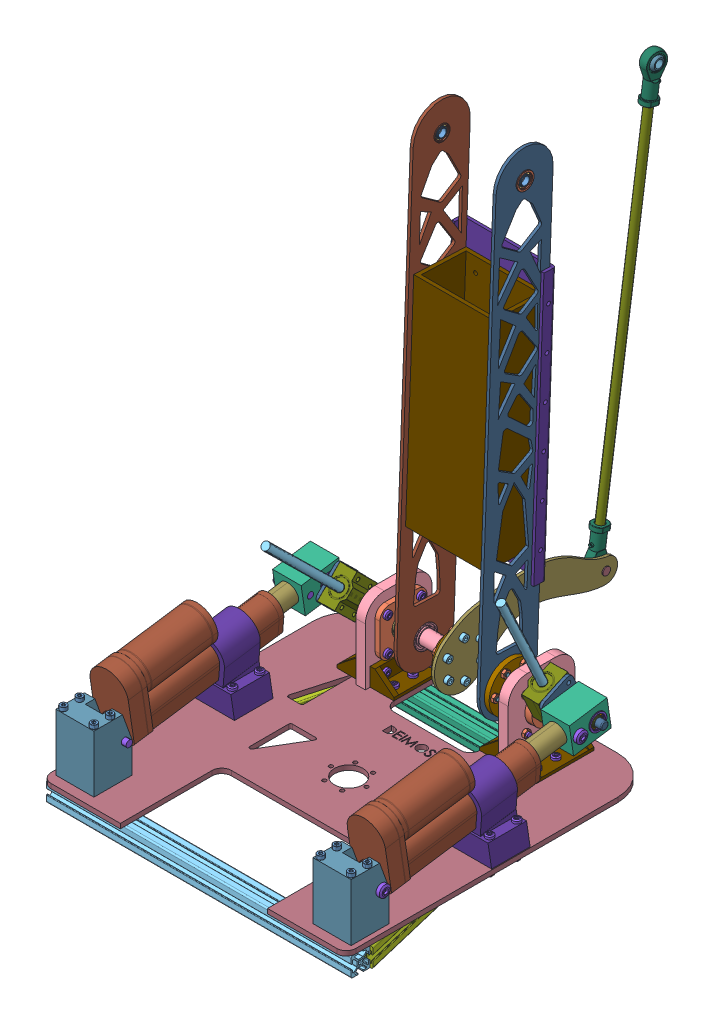
SolidWorks assembly Base + Link1 Final assembly, configuration Default. Lengths in mm. (continued)
Components (placement in the parent): (continued)
- socket head cap screw_iso-13: socket head cap screw_iso [ISO 4762 M4 x 12 - 12N] at (285.0714 147.0946 166.2039) x (-1 0 0) z (0 0.924225 0.381849) size (16 7 7)
- hex nut style 1 gradeab_iso-50: hex nut style 1 gradeab_iso [ISO - 4032 - M4 - W - N] at (269.8714 148.1762 131.5798) x (0 0 1) z (-1 0 0) size (7 8.08 3.2)
- hex nut style 1 gradeab_iso-51: hex nut style 1 gradeab_iso [ISO - 4032 - M4 - W - N] at (269.8714 157.6305 149.2041) x (0 0 1) z (-1 0 0) size (7 8.08 3.2)
- hex nut style 1 gradeab_iso-52: hex nut style 1 gradeab_iso [ISO - 4032 - M4 - W - N] at (269.8714 147.0946 166.2039) x (0 0 1) z (-1 0 0) size (7 8.08 3.2)
- hex nut style 1 gradeab_iso-53: hex nut style 1 gradeab_iso [ISO - 4032 - M4 - W - N] at (269.8714 127.1043 165.5794) x (0 0 1) z (-1 0 0) size (7 8.08 3.2)
- hex nut style 1 gradeab_iso-54: hex nut style 1 gradeab_iso [ISO - 4032 - M4 - W - N] at (269.8714 117.65 147.9551) x (0 0 1) z (-1 0 0) size (7 8.08 3.2)
- hex nut style 1 gradeab_iso-55: hex nut style 1 gradeab_iso [ISO - 4032 - M4 - W - N] at (269.8714 128.186 130.9553) x (0 0 1) z (-1 0 0) size (7 8.08 3.2)
- hex nut style 1 gradeab_iso-56: hex nut style 1 gradeab_iso [ISO - 4032 - M4 - W - N] at (336.7714 154.5674 137.9272) x (0 0 -1) z (1 0 0) size (7 8.08 3.2)
- hex nut style 1 gradeab_iso-57: hex nut style 1 gradeab_iso [ISO - 4032 - M4 - W - N] at (336.7714 136.8786 128.5941) x (0 0 -1) z (1 0 0) size (7 8.08 3.2)
- hex nut style 1 gradeab_iso-58: hex nut style 1 gradeab_iso [ISO - 4032 - M4 - W - N] at (336.7714 155.329 157.9127) x (0 0 -1) z (1 0 0) size (7 8.08 3.2)
- hex nut style 1 gradeab_iso-59: hex nut style 1 gradeab_iso [ISO - 4032 - M4 - W - N] at (336.7714 119.9515 139.2465) x (0 0 -1) z (1 0 0) size (7 8.08 3.2)
- hex nut style 1 gradeab_iso-60: hex nut style 1 gradeab_iso [ISO - 4032 - M4 - W - N] at (336.7714 120.7132 159.232) x (0 0 -1) z (1 0 0) size (7 8.08 3.2)
- hex nut style 1 gradeab_iso-61: hex nut style 1 gradeab_iso [ISO - 4032 - M4 - W - N] at (336.7714 138.4019 168.5651) x (0 0 -1) z (1 0 0) size (7 8.08 3.2)
Mates (geometry in assembly coordinates):
- Coincident12: coincident anti-aligned: plane of V8_base plate for LAURC 2024_V4-1 through (283.5714 92.6403 412.2334) normal (0 1 0); plane of LA_back holder-1 through (148.5714 92.6403 403.5796) normal (0 -1 0)
- Concentric4: concentric anti-aligned: cylinder of Connector to Linear bearing-1/V8_F688ZZ_assemblyURC 2024_V4-2/V8_F688ZZ_shaftURC 2024_V4-1 through (137.4714 160.303 171.5672) axis (-1 0 0) radius 4; cylinder of V8_bearing and cam connection_for_v4URC 2024_V4 laser cut-1 through (125.6714 160.303 171.5672) axis (1 0 0) radius 4
- Distance6: distance = 20 mm: cylinder of Connector to Linear bearing-1/V8_connectorURC 2024_V4-1 through (168.5714 167.5156 156.635) axis (0 -0.146923 0.989148) radius 13; plane of V8_bearing and cam connection_for_v4URC 2024_V4-1 through (188.5714 161.6723 163.3962) normal (-1 0 0)
- Concentric7: concentric aligned: cylinder of V8_LA_Body_V4-1 through (148.5714 127.7454 390.7229) axis (0 0.146946 -0.989144) radius 10; cylinder of V8_LA_RodURC 2024_V4-1 through (148.5714 140.671 303.7169) axis (0 0.146946 -0.989144) radius 10
- Parallel7: parallel aligned: plane of V8_bearing and cam connection_for_v4URC 2024_V4 laser cut-1 through (170.6714 137.31 173.1714) normal (-1 0 0); plane of V8_base plate for LAURC 2024_V4-1 through (123.5714 92.6403 412.2334) normal (-1 0 0)
- Coincident16: coincident anti-aligned: plane of V8_LA_Body_V4-1 through (139.5714 133.2418 401.3618) normal (-1 0 0); plane of LA_back holder-1 through (139.5714 102.6403 403.5796) normal (1 0 0)
- Concentric13: concentric aligned: cylinder of V8_LA_Body_V4-1 through (166.0567 127.6403 391.4309) axis (-1 0 0) radius 3; cylinder of LA_back holder-1 through (196.5714 127.6403 391.4309) axis (-1 0 0) radius 3
- Concentric14: concentric aligned: cylinder of linnear rod coupler-1 through (184.8714 146.065 157.125) axis (0 -0.702057 -0.712121) radius 4; cylinder of linear guid rod-1 through (184.8714 247.1612 259.6704) axis (0 -0.702057 -0.712121) radius 4
- Concentric15: concentric: cylinder of base bearing assambly-1/base shaft bearing housing-1 through (214.5714 142.6403 150.9703) axis (-1 0 0) radius 17; cylinder of V8_bearing holder holderURC 2024_V4-1 through (223.5714 142.6403 150.9703) axis (1 0 0) radius 17.5
- Coincident19: coincident anti-aligned: plane of V8_bearing holder holderURC 2024_V4-1 through (203.5714 92.6403 113.5796) normal (0 -1 0); plane of V8_base plate for LAURC 2024_V4-1 through (283.5714 92.6403 412.2334) normal (0 1 0)
- Concentric21: concentric aligned: cylinder of V8_LA_Body_V4-1 through (166.0567 127.6403 391.4309) axis (-1 0 0) radius 3; cylinder of LA_back holder-1 through (196.5714 127.6403 391.4309) axis (-1 0 0) radius 3
- Concentric24: concentric anti-aligned: cylinder of V8_base plate for LAURC 2024_V4-1 through (132.5714 82.6403 419.5796) axis (0 1 0) radius 2; cylinder of LA_back holder-1 through (132.5714 180.6403 419.5796) axis (0 -1 0) radius 2
- Concentric25: concentric anti-aligned: cylinder of V8_base plate for LAURC 2024_V4-1 through (164.5714 82.6403 419.5796) axis (0 1 0) radius 2; cylinder of LA_back holder-1 through (164.5714 180.6403 419.5796) axis (0 -1 0) radius 2
- Concentric26: concentric aligned: cylinder of Connector to Linear bearing-2/V8_F688ZZ_assemblyURC 2024_V4-2/V8_F688ZZ_shaftURC 2024_V4-1 through (407.4714 162.026 159.969) axis (-1 0 0) radius 4; cylinder of V8_bearing and cam connection_for_v4URC 2024_V4 laser cut-2 through (441.4714 162.026 159.969) axis (-1 0 0) radius 4
- Concentric31: concentric aligned: cylinder of V8_LA_RodURC 2024_V4-2 through (418.5714 142.394 292.1187) axis (0 0.146946 -0.989144) radius 10; cylinder of V8_LA_Body_V4-2 through (418.5714 127.7454 390.7229) axis (0 0.146946 -0.989144) radius 10
- Concentric36: concentric aligned: cylinder of linnear rod coupler-2 through (382.2714 148.5129 153.6577) axis (0 -0.906049 -0.423172) radius 4; cylinder of linear guid rod-2 through (382.2714 269.4957 210.1629) axis (0 -0.906049 -0.423172) radius 4
- Concentric37: concentric anti-aligned: cylinder of base bearing assambly-2/base shaft bearing housing-1 through (370.5714 137.6403 148.5796) axis (1 0 0) radius 17; cylinder of V8_bearing holder holderURC 2024_V4-2 through (363.5714 137.6403 148.5796) axis (-1 0 0) radius 17.5
- Coincident30: coincident anti-aligned: plane of linnear rod coupler-2 through (396.2714 137.6403 148.5796) normal (1 0 0); plane of lock_nut_for coupler-2 through (396.2714 137.6403 148.5796) normal (-1 0 0)
- Coincident31: coincident anti-aligned: plane of V8_base plate for LAURC 2024_V4-1 through (283.5714 92.6403 412.2334) normal (0 1 0); plane of LA_back holder-2 through (418.5714 92.6403 403.5796) normal (0 -1 0)
- Parallel13: parallel aligned: plane of V8_base plate for LAURC 2024_V4-1 through (443.5714 92.6403 412.2334) normal (1 0 0); plane of V8_bearing and cam connection_for_v4URC 2024_V4 laser cut-2 through (396.4714 168.2112 182.1724) normal (1 0 0)
- Coincident32: coincident anti-aligned: plane of V8_base plate for LAURC 2024_V4-1 through (283.5714 92.6403 412.2334) normal (0 1 0); plane of V8_bearing holder holderURC 2024_V4-2 through (363.5714 92.6403 183.5796) normal (0 -1 0)
- Concentric42: concentric anti-aligned: cylinder of V8_base plate for LAURC 2024_V4-1 through (402.5714 82.6403 419.5796) axis (0 1 0) radius 2; cylinder of LA_back holder-2 through (402.5714 180.6403 419.5796) axis (0 -1 0) radius 2
- Concentric43: concentric anti-aligned: cylinder of V8_base plate for LAURC 2024_V4-1 through (434.5714 82.6403 419.5796) axis (0 1 0) radius 2; cylinder of LA_back holder-2 through (434.5714 180.6403 419.5796) axis (0 -1 0) radius 2
- Coincident41: coincident anti-aligned: plane of LA_back holder-2 through (427.5714 102.6403 403.5796) normal (-1 0 0); plane of V8_LA_Body_V4-2 through (427.5714 133.2418 401.3618) normal (1 0 0)
- Concentric60: concentric aligned: cylinder of LA_back holder-2 through (466.5714 127.6403 391.4309) axis (-1 0 0) radius 3; cylinder of V8_LA_Body_V4-2 through (436.0567 127.6403 391.4309) axis (-1 0 0) radius 3
- Coincident46: coincident anti-aligned: plane of V8_bearing and cam connection_for_v4URC 2024_V4 laser cut-2 through (393.4714 168.2112 182.1724) normal (-1 0 0); plane of linear bearing robotic arm-2 through (393.4714 185.0413 170.7184) normal (1 0 0)
- Concentric65: concentric anti-aligned: cylinder of V8_bearing and cam connection_for_v4URC 2024_V4 laser cut-2 through (403.4714 148.7935 167.033) axis (-1 0 0) radius 2; cylinder of linear bearing robotic arm-2 through (385.4714 148.7935 167.033) axis (1 0 0) radius 1.7
- Concentric66: concentric anti-aligned: cylinder of V8_bearing and cam connection_for_v4URC 2024_V4 laser cut-2 through (403.4714 165.1024 174.6501) axis (-1 0 0) radius 2; cylinder of linear bearing robotic arm-2 through (385.4714 165.1024 174.6501) axis (1 0 0) radius 1.7
- Coincident47: coincident anti-aligned: plane of V8_bearing and cam connection_for_v4URC 2024_V4 laser cut-1 through (173.6714 137.31 173.1714) normal (1 0 0); plane of linear bearing robotic arm-1 through (173.6714 142.4694 153.478) normal (-1 0 0)
- Concentric67: concentric aligned: cylinder of V8_bearing and cam connection_for_v4URC 2024_V4 laser cut-1 through (163.6714 175.167 169.5516) axis (1 0 0) radius 2; cone of linear bearing robotic arm-1 through (173.7714 175.167 169.5516) axis (1 0 0)
- Concentric68: concentric aligned: cylinder of V8_bearing and cam connection_for_v4URC 2024_V4 laser cut-1 through (163.6714 162.5299 156.7334) axis (1 0 0) radius 2; cone of linear bearing robotic arm-1 through (173.7714 162.5299 156.7334) axis (1 0 0)
- Concentric69: concentric anti-aligned: cylinder of linear guid rod-2 through (382.2714 269.4957 210.1629) axis (0 -0.906049 -0.423172) radius 4; cylinder of linear bearing robotic arm-2 through (382.2714 148.4352 153.6214) axis (0 0.906049 0.423172) radius 4
- Concentric70: concentric aligned: cylinder of linear guid rod-1 through (184.8714 247.1612 259.6704) axis (0 -0.702057 -0.712121) radius 4; cylinder of linear bearing robotic arm-1 through (184.8714 170.8339 182.249) axis (0 -0.702057 -0.712121) radius 4
- Concentric73: concentric anti-aligned: cylinder of V8_LA_Body_V4-2 through (418.5714 153.3559 218.3306) axis (0 -0.146946 0.989144) radius 14.0003; cylinder of linear_acutator_holder-1 through (418.5714 143.3537 285.6586) axis (0 0.146946 -0.989144) radius 13.9658
- Concentric74: concentric anti-aligned: cylinder of Connector to Linear bearing-2/V8_connectorURC 2024_V4-1 through (418.5714 160.1892 172.3333) axis (0 -0.146946 0.989144) radius 10; cylinder of V8_LA_RodURC 2024_V4-2 through (418.5714 142.394 292.1187) axis (0 0.146946 -0.989144) radius 10
- Concentric76: concentric anti-aligned: cylinder of Connector to Linear bearing-2/V8_connectorURC 2024_V4-1 through (504.5714 159.1459 179.3562) axis (-1 0 0) radius 3; cylinder of V8_LA_RodURC 2024_V4-2 through (408.5704 159.1459 179.3562) axis (1 0 0) radius 3
- Concentric77: concentric anti-aligned: cylinder of Connector to Linear bearing-1/V8_connectorURC 2024_V4-1 through (148.5714 158.4662 183.9315) axis (0 -0.146946 0.989144) radius 10; cylinder of V8_LA_RodURC 2024_V4-1 through (148.5714 140.671 303.7169) axis (0 0.146946 -0.989144) radius 10
- Concentric78: concentric anti-aligned: cylinder of Connector to Linear bearing-1/V8_connectorURC 2024_V4-1 through (234.5714 157.4228 190.9544) axis (-1 0 0) radius 3; cylinder of V8_LA_RodURC 2024_V4-1 through (138.5704 157.4228 190.9544) axis (1 0 0) radius 3
- Coincident51: coincident anti-aligned: plane of V8_base plate for LAURC 2024_V4-1 through (283.5714 92.6403 412.2334) normal (0 1 0); plane of linear_acutator_holder-2 through (124.6971 92.6403 239.7077) normal (0 -1 0)
- Concentric79: concentric anti-aligned: cylinder of V8_LA_Body_V4-1 through (148.5714 153.3559 218.3306) axis (0 -0.146946 0.989144) radius 14.0003; cylinder of linear_acutator_holder-2 through (148.5714 143.3537 285.6586) axis (0 0.146946 -0.989144) radius 18.9535
- Concentric80: concentric anti-aligned: cylinder of base bearing assambly-2/base shaft bearing housing-1 through (358.5714 155.1403 131.0796) axis (-1 0 0) radius 2; cylinder of V8_bearing holder holderURC 2024_V4-2 through (353.5714 155.1403 131.0796) axis (1 0 0) radius 2
- Coincident52: coincident anti-aligned: plane of V8_bearing holder holderURC 2024_V4-2 through (363.5714 172.6403 183.5796) normal (1 0 0); plane of l bracket_arm base flang-1 through (363.5714 111.6403 178.5796) normal (-1 0 0)
- Coincident53: coincident anti-aligned: plane of V8_base plate for LAURC 2024_V4-1 through (283.5714 92.6403 412.2334) normal (0 1 0); plane of l bracket_arm base flang-1 through (368.5714 92.6403 178.5796) normal (0 -1 0)
- Width1: width anti-aligned: plane of l bracket_arm base flang-1 through (368.5714 111.6403 178.5796) normal (0 0 1); plane of V8_bearing holder holderURC 2024_V4-2 through (368.5714 111.6403 118.5796) normal (0 0 -1); plane of l bracket_arm base flang-1 through (363.5714 172.6403 113.5796) normal (0 0 -1); plane of V8_bearing holder holderURC 2024_V4-2 through (363.5714 172.6403 183.5796) normal (0 0 1)
- Coincident55: coincident anti-aligned: plane of V8_base plate for LAURC 2024_V4-1 through (283.5714 92.6403 412.2334) normal (0 1 0); plane of l bracket_arm base flang-2 through (348.5714 92.6403 118.5796) normal (0 -1 0)
- Coincident56: coincident anti-aligned: plane of V8_bearing holder holderURC 2024_V4-2 through (353.5714 172.6403 183.5796) normal (-1 0 0); plane of l bracket_arm base flang-2 through (353.5714 111.6403 118.5796) normal (1 0 0)
- Coincident57: coincident aligned: plane of l bracket_arm base flang-1 through (368.5714 111.6403 118.5796) normal (0 0 -1); plane of l bracket_arm base flang-2 through (348.5714 111.6403 118.5796) normal (0 0 -1)
- Concentric81: concentric anti-aligned: cylinder of base bearing assambly-2/base shaft bearing housing-1 through (370.5714 137.6403 148.5796) axis (1 0 0) radius 17; cylinder of V8_bearing holder holderURC 2024_V4-2 through (363.5714 137.6403 148.5796) axis (-1 0 0) radius 17.5
- Coincident59: coincident anti-aligned: plane of base bearing assambly-2/base shaft bearing housing-1 through (353.5714 172.6403 148.5796) normal (1 0 0); plane of V8_bearing holder holderURC 2024_V4-2 through (353.5714 172.6403 183.5796) normal (-1 0 0)
- Concentric83: concentric anti-aligned: cylinder of base bearing assambly-1/base shaft bearing housing-1 through (196.5714 137.6403 148.5796) axis (-1 0 0) radius 17; cylinder of V8_bearing holder holderURC 2024_V4-1 through (203.5714 137.6403 148.5796) axis (1 0 0) radius 17.5
- Coincident60: coincident aligned: plane of l bracket_arm base flang-2 through (348.5714 111.6403 118.5796) normal (0 0 -1); plane of l bracket_arm base flang-4 through (218.5714 111.6403 118.5796) normal (0 0 -1)
- Coincident61: coincident anti-aligned: plane of V8_bearing holder holderURC 2024_V4-1 through (213.5714 172.6403 113.5796) normal (1 0 0); plane of l bracket_arm base flang-4 through (213.5714 111.6403 178.5796) normal (-1 0 0)
- Coincident62: coincident anti-aligned: plane of V8_base plate for LAURC 2024_V4-1 through (283.5714 92.6403 412.2334) normal (0 1 0); plane of l bracket_arm base flang-4 through (218.5714 92.6403 178.5796) normal (0 -1 0)
- Coincident63: coincident anti-aligned: plane of V8_bearing holder holderURC 2024_V4-1 through (203.5714 172.6403 113.5796) normal (-1 0 0); plane of l bracket_arm base flang-3 through (203.5714 111.6403 118.5796) normal (1 0 0)
- Coincident64: coincident anti-aligned: plane of V8_base plate for LAURC 2024_V4-1 through (283.5714 92.6403 412.2334) normal (0 1 0); plane of l bracket_arm base flang-3 through (198.5714 92.6403 118.5796) normal (0 -1 0)
- Coincident65: coincident aligned: plane of l bracket_arm base flang-3 through (198.5714 111.6403 118.5796) normal (0 0 -1); plane of l bracket_arm base flang-4 through (218.5714 111.6403 118.5796) normal (0 0 -1)
- Coincident66: coincident aligned: plane of V8_base plate for LAURC 2024_V4-1 through (328.5714 97.6403 188.5796) normal (-1 0 0); plane of l bracket_arm base flang-2 through (328.5714 111.6403 118.5796) normal (-1 0 0)
- Coincident67: coincident aligned: plane of V8_base plate for LAURC 2024_V4-1 through (238.5714 97.6403 108.5796) normal (1 0 0); plane of l bracket_arm base flang-4 through (238.5714 111.6403 178.5796) normal (1 0 0)
- Parallel17: parallel anti-aligned: plane of V8_LA_Body_V4-2 through (428.5714 112.1188 359.8068) normal (0 -0.989144 -0.146946); plane of linear_acutator_holder-1 through (408.5961 123.6195 282.7269) normal (0 0.989144 0.146946)
- Coincident72: coincident: line of V8_base plate for LAURC 2024_V4-1 through (238.5714 87.6403 118.5796) axis (0 1 0); plane of l bracket_arm base flang-4 through (218.5714 111.6403 118.5796) normal (0 0 -1)
- Distance14: distance = 6 mm anti-aligned: plane of V8_bearing and cam connection_for_v4URC 2024_V4 laser cut-2 through (396.4714 168.2112 182.1724) normal (1 0 0); plane of Connector to Linear bearing-2/V8_F688ZZ_assemblyURC 2024_V4-2/V8_F688ZZ_HousingURC 2024_V4-1 through (402.4714 162.026 159.969) normal (-1 0 0)
- Distance16: distance = 6 mm anti-aligned: plane of V8_bearing and cam connection_for_v4URC 2024_V4 laser cut-1 through (170.6714 137.31 173.1714) normal (-1 0 0); plane of Connector to Linear bearing-1/V8_F688ZZ_assemblyURC 2024_V4-1/V8_F688ZZ_HousingURC 2024_V4-1 through (164.6714 160.303 171.5672) normal (1 0 0)
- Coincident76: coincident anti-aligned: plane of base bearing assambly-1/base shaft bearing housing-1 through (213.5714 172.6403 148.5796) normal (-1 0 0); plane of V8_bearing holder holderURC 2024_V4-1 through (213.5714 172.6403 113.5796) normal (1 0 0)
- Concentric84: concentric anti-aligned: cylinder of base bearing assambly-1/base shaft bearing housing-1 through (208.5714 155.1403 166.0796) axis (1 0 0) radius 2; cylinder of V8_bearing holder holderURC 2024_V4-1 through (213.5714 155.1403 166.0796) axis (-1 0 0) radius 2
- Concentric91: concentric aligned: cylinder of LA_back holder-2 through (402.5714 180.6403 419.5796) axis (0 -1 0) radius 2; cylinder of Screw_DIN_912_M4x70_A2.step-1 through (402.5714 102.6403 419.5796) axis (0 -1 0) radius 2
- Coincident83: coincident anti-aligned: plane of LA_back holder-2 through (418.5714 152.6403 403.5796) normal (0 1 0); plane of Screw_DIN_912_M4x70_A2.step-1 through (402.5714 152.6403 419.5796) normal (0 -1 0)
- Concentric92: concentric aligned: cylinder of LA_back holder-2 through (434.5714 180.6403 419.5796) axis (0 -1 0) radius 2; cylinder of Screw_DIN_912_M4x70_A2.step-2 through (434.5714 102.6403 419.5796) axis (0 -1 0) radius 2
- Coincident84: coincident anti-aligned: plane of LA_back holder-2 through (418.5714 152.6403 403.5796) normal (0 1 0); plane of Screw_DIN_912_M4x70_A2.step-2 through (434.5714 152.6403 419.5796) normal (0 -1 0)
- Concentric93: concentric aligned: cylinder of LA_back holder-2 through (434.5714 180.6403 402.6026) axis (0 -1 0) radius 2; cylinder of Screw_DIN_912_M4x70_A2.step-4 through (434.5714 102.6403 402.6026) axis (0 -1 0) radius 2
- Coincident85: coincident anti-aligned: plane of LA_back holder-2 through (418.5714 152.6403 403.5796) normal (0 1 0); plane of Screw_DIN_912_M4x70_A2.step-4 through (434.5714 152.6403 402.6026) normal (0 -1 0)
- Concentric94: concentric aligned: cylinder of LA_back holder-2 through (402.5714 180.6403 402.6026) axis (0 -1 0) radius 2; cylinder of Screw_DIN_912_M4x70_A2.step-6 through (402.5714 102.6403 402.6026) axis (0 -1 0) radius 2
- Coincident86: coincident anti-aligned: plane of LA_back holder-2 through (418.5714 152.6403 403.5796) normal (0 1 0); plane of Screw_DIN_912_M4x70_A2.step-6 through (402.5714 152.6403 402.6026) normal (0 -1 0)
- Concentric95: concentric aligned: cylinder of LA_back holder-1 through (164.5714 180.6403 419.5796) axis (0 -1 0) radius 2; cylinder of Screw_DIN_912_M4x70_A2.step-8 through (164.5714 102.6403 419.5796) axis (0 -1 0) radius 2
- Coincident87: coincident anti-aligned: plane of LA_back holder-1 through (148.5714 152.6403 403.5796) normal (0 1 0); plane of Screw_DIN_912_M4x70_A2.step-8 through (164.5714 152.6403 419.5796) normal (0 -1 0)
- Concentric96: concentric aligned: cylinder of LA_back holder-1 through (164.5714 180.6403 402.6026) axis (0 -1 0) radius 2; cylinder of Screw_DIN_912_M4x70_A2.step-10 through (164.5714 102.6403 402.6026) axis (0 -1 0) radius 2
- Coincident88: coincident anti-aligned: plane of LA_back holder-1 through (148.5714 152.6403 403.5796) normal (0 1 0); plane of Screw_DIN_912_M4x70_A2.step-10 through (164.5714 152.6403 402.6026) normal (0 -1 0)
- Concentric97: concentric aligned: cylinder of LA_back holder-1 through (132.5714 180.6403 419.5796) axis (0 -1 0) radius 2; cylinder of Screw_DIN_912_M4x70_A2.step-12 through (132.5714 102.6403 419.5796) axis (0 -1 0) radius 2
- Coincident89: coincident anti-aligned: plane of LA_back holder-1 through (148.5714 152.6403 403.5796) normal (0 1 0); plane of Screw_DIN_912_M4x70_A2.step-12 through (132.5714 152.6403 419.5796) normal (0 -1 0)
- Concentric98: concentric aligned: cylinder of LA_back holder-1 through (132.5714 180.6403 402.6026) axis (0 -1 0) radius 2; cylinder of Screw_DIN_912_M4x70_A2.step-14 through (132.5714 102.6403 402.6026) axis (0 -1 0) radius 2
- Coincident90: coincident anti-aligned: plane of LA_back holder-1 through (148.5714 152.6403 403.5796) normal (0 1 0); plane of Screw_DIN_912_M4x70_A2.step-14 through (132.5714 152.6403 402.6026) normal (0 -1 0)
- Concentric99: concentric anti-aligned: cylinder of V8_base plate for LAURC 2024_V4-1 through (402.5714 82.6403 419.5796) axis (0 1 0) radius 2; cylinder of hex nut style 1 gradeab_iso-8 through (402.5714 87.6403 419.5796) axis (0 -1 0) radius 1.65
- Coincident91: coincident anti-aligned: plane of V8_base plate for LAURC 2024_V4-1 through (283.5714 87.6403 412.2334) normal (0 -1 0); plane of hex nut style 1 gradeab_iso-8 through (395.5728 87.6403 419.4444) normal (0 1 0)
- Concentric100: concentric anti-aligned: cylinder of V8_base plate for LAURC 2024_V4-1 through (434.5714 82.6403 419.5796) axis (0 1 0) radius 2; cylinder of hex nut style 1 gradeab_iso-9 through (434.5714 87.6403 419.5796) axis (0 -1 0) radius 1.65
- Coincident92: coincident anti-aligned: plane of V8_base plate for LAURC 2024_V4-1 through (283.5714 87.6403 412.2334) normal (0 -1 0); plane of hex nut style 1 gradeab_iso-9 through (427.6727 87.6403 420.7658) normal (0 1 0)
- Concentric101: concentric aligned: circle of Screw_DIN_912_M4x70_A2.step-4; cylinder of hex nut style 1 gradeab_iso-11 through (434.5714 87.6403 402.6026) axis (0 -1 0) radius 1.65
- Coincident93: coincident anti-aligned: plane of V8_base plate for LAURC 2024_V4-1 through (283.5714 87.6403 412.2334) normal (0 -1 0); plane of hex nut style 1 gradeab_iso-11 through (430.6304 87.6403 408.3878) normal (0 1 0)
- Concentric102: concentric aligned: circle of Screw_DIN_912_M4x70_A2.step-6; cylinder of hex nut style 1 gradeab_iso-14 through (402.5714 87.6403 402.6026) axis (0 -1 0) radius 1.65
- Coincident94: coincident anti-aligned: plane of V8_base plate for LAURC 2024_V4-1 through (283.5714 87.6403 412.2334) normal (0 -1 0); plane of hex nut style 1 gradeab_iso-14 through (398.6304 87.6403 408.3878) normal (0 1 0)
- Concentric103: concentric anti-aligned: circle of V8_base plate for LAURC 2024_V4-1; cylinder of hex nut style 1 gradeab_iso-16 through (164.5714 87.6403 419.5796) axis (0 -1 0) radius 1.65
- Coincident95: coincident anti-aligned: plane of V8_base plate for LAURC 2024_V4-1 through (283.5714 87.6403 412.2334) normal (0 -1 0); plane of hex nut style 1 gradeab_iso-16 through (160.0326 87.6403 424.9087) normal (0 1 0)
- Concentric104: concentric aligned: circle of Screw_DIN_912_M4x70_A2.step-10; cylinder of hex nut style 1 gradeab_iso-18 through (164.5714 87.6403 402.6026) axis (0 -1 0) radius 1.65
- Coincident96: coincident anti-aligned: plane of V8_base plate for LAURC 2024_V4-1 through (283.5714 87.6403 412.2334) normal (0 -1 0); plane of hex nut style 1 gradeab_iso-18 through (160.6304 87.6403 408.3878) normal (0 1 0)
- Concentric105: concentric aligned: circle of Screw_DIN_912_M4x70_A2.step-12; cylinder of hex nut style 1 gradeab_iso-20 through (132.5714 87.6403 419.5796) axis (0 -1 0) radius 1.65
- Coincident97: coincident anti-aligned: plane of V8_base plate for LAURC 2024_V4-1 through (283.5714 87.6403 412.2334) normal (0 -1 0); plane of hex nut style 1 gradeab_iso-20 through (128.6304 87.6403 425.3648) normal (0 1 0)
- Concentric106: concentric aligned: circle of Screw_DIN_912_M4x70_A2.step-14; cylinder of hex nut style 1 gradeab_iso-22 through (132.5714 87.6403 402.6026) axis (0 -1 0) radius 1.65
- Coincident98: coincident anti-aligned: plane of V8_base plate for LAURC 2024_V4-1 through (283.5714 87.6403 412.2334) normal (0 -1 0); plane of hex nut style 1 gradeab_iso-22 through (128.6304 87.6403 408.3878) normal (0 1 0)
- Concentric107: concentric aligned: circle of linnear rod coupler-2; circle of lock_nut_for coupler-2
- Concentric108: concentric aligned: circle of lock_nut_for coupler-2; cylinder of base bearing assambly-2/base shaft bearing housing-1 through (370.5714 137.6403 148.5796) axis (1 0 0) radius 8
- Coincident100: coincident anti-aligned: plane of V8_base plate for LAURC 2024_V4-1 through (283.5714 92.6403 412.2334) normal (0 1 0); plane of linear_acutator_holder-1 through (394.6971 92.6403 239.7077) normal (0 -1 0)
- Tangent2: tangent: cylinder of linnear rod coupler-2 through (388.2714 137.6403 148.5796) axis (-1 0 0) radius 6; circle of linear guid rod-2
- Tangent3: tangent: cylinder of linnear rod coupler-1 through (178.8714 137.6403 148.5796) axis (1 0 0) radius 6; circle of linear guid rod-1
- Concentric109: concentric anti-aligned: cylinder of linnear rod coupler-1 through (178.8714 137.6403 148.5796) axis (1 0 0) radius 6; cylinder of base bearing assambly-1/base shaft bearing housing-1 through (196.5714 137.6403 148.5796) axis (-1 0 0) radius 8
- Concentric110: concentric anti-aligned: cylinder of base bearing assambly-2/base shaft bearing housing-1 through (370.5714 137.6403 148.5796) axis (1 0 0) radius 8; cylinder of V8_shaftURC 2024_V4 real part-1 through (333.5714 137.6403 148.5796) axis (-1 0 0) radius 7.5
- Concentric111: concentric anti-aligned: cylinder of base bearing assambly-1/base shaft bearing housing-1 through (196.5714 137.6403 148.5796) axis (-1 0 0) radius 8; cylinder of V8_shaftURC 2024_V4-1 through (273.0714 137.6403 148.5796) axis (1 0 0) radius 7.5
- Coincident102: coincident aligned: plane of V8_bearing holder holderURC 2024_V4-1 through (203.5714 172.6403 113.5796) normal (0 0 -1); plane of V8_bearing holder holderURC 2024_V4-2 through (363.5714 172.6403 113.5796) normal (0 0 -1)
- Coincident105: coincident aligned: plane of linnear rod coupler-1 through (170.8714 137.6403 148.5796) normal (-1 0 0); plane of V8_shaftURC 2024_V4-1 through (170.8714 137.6403 148.5796) normal (-1 0 0)
- Coincident106: coincident anti-aligned: plane of V8_base plate for LAURC 2024_V4-1 through (283.5714 87.6403 412.2334) normal (0 -1 0); plane of 20 20 aluminium extrusion T slot-1 through (443.5714 87.6403 427.0796) normal (0 1 0)
- Coincident107: coincident aligned: plane of V8_base plate for LAURC 2024_V4-1 through (443.5714 92.6403 412.2334) normal (1 0 0); plane of 20 20 aluminium extrusion T slot-1 through (443.5714 74.5023 409.0876) normal (1 0 0)
- Distance17: distance = 5 mm aligned: plane of 20 20 aluminium extrusion T slot-1 through (443.5714 69.1403 428.5796) normal (0 0 1); plane of V8_base plate for LAURC 2024_V4-1 through (283.5714 92.6403 433.5796) normal (0 0 1)
- Coincident108: coincident anti-aligned: plane of V8_base plate for LAURC 2024_V4-1 through (283.5714 87.6403 412.2334) normal (0 -1 0); plane of 20 20 aluminium extrusion T slot 200 mm-1 through (383.5714 87.6403 157.0796) normal (0 1 0)
- Parallel18: parallel aligned: plane of V8_base plate for LAURC 2024_V4-1 through (443.5714 92.6403 412.2334) normal (1 0 0); plane of 20 20 aluminium extrusion T slot 200 mm-1 through (383.5714 74.5023 139.0876) normal (1 0 0)
- Coincident109: coincident anti-aligned: plane of V8_base plate for LAURC 2024_V4-1 through (283.5714 87.6403 412.2334) normal (0 -1 0); plane of 20 20 aluminium extrusion T slot at angle-1 through (383.9984 87.6403 154.2734) normal (0 1 0)
- Distance18: distance = 60 mm aligned: plane of V8_base plate for LAURC 2024_V4-1 through (443.5714 92.6403 412.2334) normal (1 0 0); plane of 20 20 aluminium extrusion T slot 200 mm-1 through (383.5714 74.5023 139.0876) normal (1 0 0)
- Coincident111: coincident anti-aligned: plane of 20 20 aluminium extrusion T slot 200 mm-1 through (383.5714 69.1403 158.5796) normal (0 0 1); plane of 20 20 aluminium extrusion T slot at angle-1 through (386.5714 87.6403 158.5796) normal (0 0 -1)
- Distance20: distance = 30 mm aligned: plane of V8_base plate for LAURC 2024_V4-1 through (283.5714 92.6403 108.5796) normal (0 0 -1); plane of 20 20 aluminium extrusion T slot 200 mm-1 through (383.5714 86.1403 138.5796) normal (0 0 -1)
- Coincident113: coincident anti-aligned: plane of 20 20 aluminium extrusion T slot 200 mm-1 through (383.5714 69.1403 158.5796) normal (0 0 1); plane of 20 20 aluminium extrusion T slot at angle-2 through (201.1363 67.6403 158.5796) normal (0 0 -1)
- Parallel19: parallel anti-aligned: plane of 20 20 aluminium extrusion T slot-1 through (443.5714 74.5023 408.5796) normal (0 0 -1); plane of 20 20 aluminium extrusion T slot at angle-2 through (141.3123 67.6403 408.5333) normal (0 0 1)
- Coincident115: coincident anti-aligned: plane of V8_base plate for LAURC 2024_V4-1 through (283.5714 87.6403 412.2334) normal (0 -1 0); plane of 20 20 aluminium extrusion T slot at angle-2 through (122.2062 87.6403 408.8825) normal (0 1 0)
- Distance21: distance = 3 mm aligned: line of 20 20 aluminium extrusion T slot at angle-2 through (180.5714 69.1403 158.5796) axis (0 1 0); line of 20 20 aluminium extrusion T slot 200 mm-1 through (183.5714 69.1403 158.5796) axis (0 1 0)
- Lock1: lock: 
- Concentric112: concentric anti-aligned: cylinder of l bracket_arm base flang-1 through (378.5714 90.6403 168.5796) axis (0 1 0) radius 2; cylinder of hexalobular socket pan head_iso-2 through (378.5714 83.6403 168.5796) axis (0 -1 0) radius 2.35
- Coincident116: coincident anti-aligned: plane of l bracket_arm base flang-1 through (388.5714 95.6403 178.5796) normal (0 1 0); plane of hexalobular socket pan head_iso-2 through (380.9214 95.6403 168.5796) normal (0 -1 0)
- Concentric113: concentric anti-aligned: cylinder of l bracket_arm base flang-1 through (378.5714 90.6403 148.5796) axis (0 1 0) radius 2; cylinder of hexalobular socket pan head_iso-3 through (378.5714 83.6403 148.5796) axis (0 -1 0) radius 2.35
- Coincident117: coincident anti-aligned: plane of l bracket_arm base flang-1 through (388.5714 95.6403 178.5796) normal (0 1 0); plane of hexalobular socket pan head_iso-3 through (380.9214 95.6403 148.5796) normal (0 -1 0)
- Concentric114: concentric anti-aligned: cylinder of l bracket_arm base flang-1 through (378.5714 90.6403 128.5796) axis (0 1 0) radius 2; cylinder of hexalobular socket pan head_iso-4 through (378.5714 83.6403 128.5796) axis (0 -1 0) radius 2.35
- Coincident118: coincident anti-aligned: plane of l bracket_arm base flang-1 through (388.5714 95.6403 178.5796) normal (0 1 0); plane of hexalobular socket pan head_iso-4 through (380.9214 95.6403 128.5796) normal (0 -1 0)
- Concentric115: concentric anti-aligned: cylinder of l bracket_arm base flang-2 through (338.5714 90.6403 168.5796) axis (0 1 0) radius 2; cylinder of hexalobular socket pan head_iso-5 through (338.5714 83.6403 168.5796) axis (0 -1 0) radius 2.35
- Coincident119: coincident anti-aligned: plane of l bracket_arm base flang-2 through (328.5714 95.6403 118.5796) normal (0 1 0); plane of hexalobular socket pan head_iso-5 through (340.9214 95.6403 168.5796) normal (0 -1 0)
- Concentric116: concentric anti-aligned: cylinder of l bracket_arm base flang-2 through (338.5714 90.6403 148.5796) axis (0 1 0) radius 2; cylinder of hexalobular socket pan head_iso-6 through (338.5714 83.6403 148.5796) axis (0 -1 0) radius 2.35
- Coincident120: coincident anti-aligned: plane of l bracket_arm base flang-2 through (328.5714 95.6403 118.5796) normal (0 1 0); plane of hexalobular socket pan head_iso-6 through (340.9214 95.6403 148.5796) normal (0 -1 0)
- Concentric117: concentric anti-aligned: cylinder of l bracket_arm base flang-2 through (338.5714 90.6403 128.5796) axis (0 1 0) radius 2; cylinder of hexalobular socket pan head_iso-7 through (338.5714 83.6403 128.5796) axis (0 -1 0) radius 2.35
- Coincident121: coincident anti-aligned: plane of l bracket_arm base flang-2 through (328.5714 95.6403 118.5796) normal (0 1 0); plane of hexalobular socket pan head_iso-7 through (340.9214 95.6403 128.5796) normal (0 -1 0)
- Concentric118: concentric anti-aligned: cylinder of l bracket_arm base flang-4 through (228.5714 90.6403 128.5796) axis (0 1 0) radius 2; cylinder of hexalobular socket pan head_iso-8 through (228.5714 83.6403 128.5796) axis (0 -1 0) radius 2.35
- Coincident122: coincident anti-aligned: plane of l bracket_arm base flang-4 through (238.5714 95.6403 178.5796) normal (0 1 0); plane of hexalobular socket pan head_iso-8 through (230.9214 95.6403 128.5796) normal (0 -1 0)
- Concentric119: concentric anti-aligned: cylinder of l bracket_arm base flang-4 through (228.5714 90.6403 148.5796) axis (0 1 0) radius 2; cylinder of hexalobular socket pan head_iso-9 through (228.5714 83.6403 148.5796) axis (0 -1 0) radius 2.35
- Coincident123: coincident anti-aligned: plane of l bracket_arm base flang-4 through (238.5714 95.6403 178.5796) normal (0 1 0); plane of hexalobular socket pan head_iso-9 through (230.9214 95.6403 148.5796) normal (0 -1 0)
- Concentric120: concentric anti-aligned: cylinder of l bracket_arm base flang-4 through (228.5714 90.6403 168.5796) axis (0 1 0) radius 2; cylinder of hexalobular socket pan head_iso-10 through (228.5714 83.6403 168.5796) axis (0 -1 0) radius 2.35
- Coincident124: coincident anti-aligned: plane of l bracket_arm base flang-4 through (238.5714 95.6403 178.5796) normal (0 1 0); plane of hexalobular socket pan head_iso-10 through (230.9214 95.6403 168.5796) normal (0 -1 0)
- Concentric121: concentric anti-aligned: cylinder of l bracket_arm base flang-3 through (188.5714 90.6403 128.5796) axis (0 1 0) radius 2; cylinder of hexalobular socket pan head_iso-11 through (188.5714 83.6403 128.5796) axis (0 -1 0) radius 2.35
- Coincident125: coincident anti-aligned: plane of l bracket_arm base flang-3 through (178.5714 95.6403 118.5796) normal (0 1 0); plane of hexalobular socket pan head_iso-11 through (190.9214 95.6403 128.5796) normal (0 -1 0)
- Concentric122: concentric anti-aligned: cylinder of l bracket_arm base flang-3 through (188.5714 90.6403 148.5796) axis (0 1 0) radius 2; cylinder of hexalobular socket pan head_iso-12 through (188.5714 83.6403 148.5796) axis (0 -1 0) radius 2.35
- Coincident126: coincident anti-aligned: plane of l bracket_arm base flang-3 through (178.5714 95.6403 118.5796) normal (0 1 0); plane of hexalobular socket pan head_iso-12 through (190.9214 95.6403 148.5796) normal (0 -1 0)
- Concentric123: concentric anti-aligned: cylinder of l bracket_arm base flang-3 through (188.5714 90.6403 168.5796) axis (0 1 0) radius 2; cylinder of hexalobular socket pan head_iso-13 through (188.5714 83.6403 168.5796) axis (0 -1 0) radius 2.35
- Coincident127: coincident anti-aligned: plane of l bracket_arm base flang-3 through (178.5714 95.6403 118.5796) normal (0 1 0); plane of hexalobular socket pan head_iso-13 through (190.9214 95.6403 168.5796) normal (0 -1 0)
- Concentric125: concentric anti-aligned: cylinder of l bracket_arm base flang-2 through (353.5714 103.6403 129.5796) axis (-1 0 0) radius 1.6729; cylinder of hexalobular socket pan head_iso-16 through (373.5714 103.6403 129.5796) axis (1 0 0) radius 2.35
- Coincident129: coincident anti-aligned: plane of l bracket_arm base flang-2 through (348.5714 111.6403 118.5796) normal (-1 0 0); plane of hexalobular socket pan head_iso-16 through (348.5714 105.9903 129.5796) normal (1 0 0)
- Concentric126: concentric anti-aligned: cylinder of l bracket_arm base flang-2 through (353.5714 103.6403 148.5796) axis (-1 0 0) radius 1.6729; cylinder of hexalobular socket pan head_iso-17 through (373.5714 103.6403 148.5796) axis (1 0 0) radius 2.35
- Coincident130: coincident anti-aligned: plane of l bracket_arm base flang-2 through (348.5714 111.6403 118.5796) normal (-1 0 0); plane of hexalobular socket pan head_iso-17 through (348.5714 105.9903 148.5796) normal (1 0 0)
- Concentric127: concentric anti-aligned: cylinder of l bracket_arm base flang-2 through (353.5714 103.6403 167.5796) axis (-1 0 0) radius 1.6729; cylinder of hexalobular socket pan head_iso-18 through (373.5714 103.6403 167.5796) axis (1 0 0) radius 2.35
- Coincident131: coincident anti-aligned: plane of l bracket_arm base flang-2 through (348.5714 111.6403 118.5796) normal (-1 0 0); plane of hexalobular socket pan head_iso-18 through (348.5714 105.9903 167.5796) normal (1 0 0)
